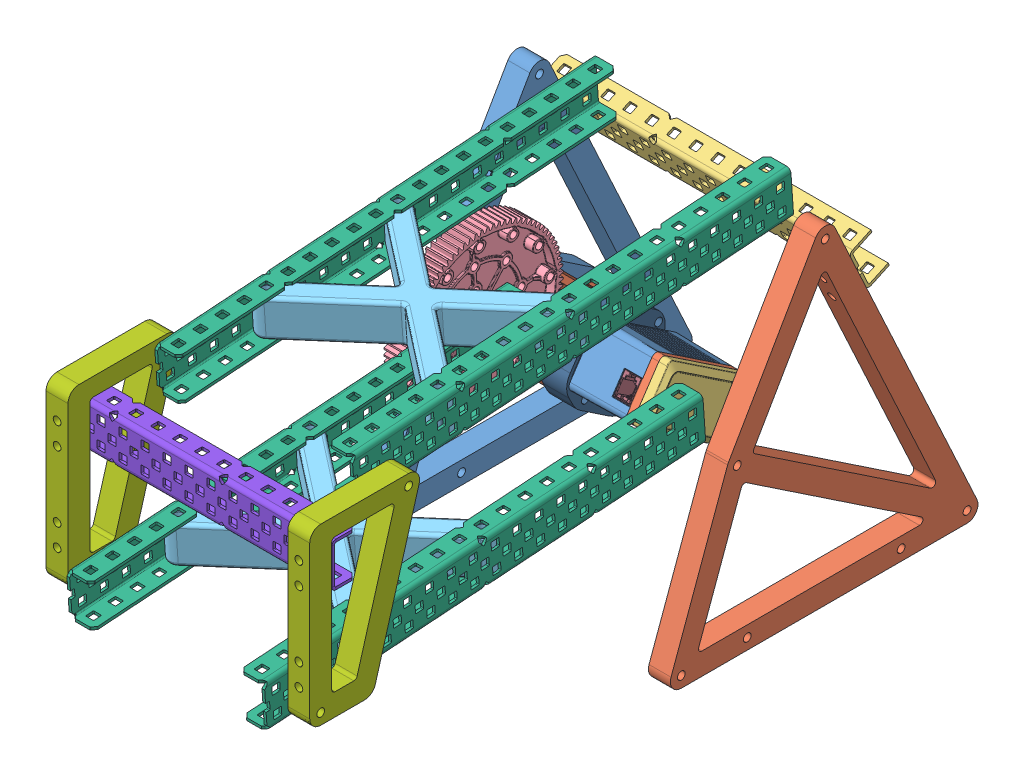
SolidWorks assembly RearArmAssembly, configuration Default. Lengths in mm.
43 component instances, 23 part files, 28 mates.
Components (placement in the parent):
- ArmMount-1: ArmMount [Default] at (3.0815 119.4615 170.9285) size (12.7 189.78 177.8)
- ArmMount(mirror)-1: ArmMount(mirror) [Default] at (168.1815 119.4615 170.9285) size (12.7 189.78 177.8)
- 1x2x1x14 Aluminum C-Channel-1: 1x2x1x14 Aluminum C-Channel [Default] at (225.3315 181.5036 101.1108) x (1 0 0) z (0 -0.420336 0.907368) size (177.8 25.41 13.97)
- RearArm_BottomBar-1: RearArm_BottomBar [Default] at (222.7102 54.1717 183.8088) x (0 -0.069828 0.997559) z (-1 0 0) size (286.79 90.98 127)
  - 84T High Strength Gear (276-3438)-1: 84T High Strength Gear (276-3438) [Default] at (-17.4079 64.2311 194.2288) size (90.98 90.98 12.7)
  - ArmXBrace-1: ArmXBrace [Default] at (128.6421 53.1059 130.7288) x (0 0 1) z (-1 0 0) size (111.86 22.25 88.94)
  - 1x2x1x20 Aluminum C-Channel-1: 1x2x1x20 Aluminum C-Channel [Default] at (192.1421 64.2311 187.8788) size (254 25.41 13.97)
  - 1x2x1x20 Aluminum C-Channel-2: 1x2x1x20 Aluminum C-Channel [Default] at (192.1421 64.2311 73.5788) x (1 0 0) z (0 0 -1) size (254 25.41 13.97)
- RearArm_TopBar-1: RearArm_TopBar [Default] at (12.5514 278.2747 177.0234) x (0 -0.069828 0.997559) z (1 0 0) size (254 25.4 114.31)
  - ArmXBrace-1: ArmXBrace [Default] at (94.2395 63.4998 79.4301) x (0 0 1) z (-1 0 0) size (111.86 22.25 88.94)
  - 1x2x1x20 Aluminum C-Channel-1: 1x2x1x20 Aluminum C-Channel [Default] at (157.7395 74.625 136.5801) size (254 25.41 13.97)
  - 1x2x1x20 Aluminum C-Channel-2: 1x2x1x20 Aluminum C-Channel [Default] at (157.7395 74.625 22.2801) x (1 0 0) z (0 0 -1) size (254 25.41 13.97)
- ArmEndAssembly-1: ArmEndAssembly [Default] at (208.3285 70.3449 488.0787) x (-1 0 0) z (0 0 -1) size (152.48 100.69 63.5)
  - ArmEnd-1: ArmEnd [Default] at (40.147 33.1539 89.1082) size (12.7 100.69 63.5)
  - ArmEnd-2: ArmEnd [Default] at (179.847 33.1539 89.1082) size (12.7 100.69 63.5)
  - 1x2x1x12 Aluminum C-Channel-1: 1x2x1x12 Aluminum C-Channel [Default] at (262.3169 103.0039 95.4582) x (1 0 0) z (0 0 -1) size (152.4 25.41 13.97)
- 0.5in 0.375in OD Nylon Spacer-1: 0.5in 0.375in OD Nylon Spacer [Default] at (22.1315 87.6603 123.4437) x (0 1 0) z (0 0 1) size (9.53 12.7 9.53)
- ArmMotorMount-1: ArmMotorMount [Default] at (41.1815 87.6603 123.4437) x (0 0.830879 -0.556452) z (1 0 0) size (48.1 53.1 15)
- 1.00_ Standoff (275-1016)-1: 1.00_ Standoff (275-1016) [Default] at (28.4815 71.832 134.0442) x (0 -1 0) z (0 0 1) size (7.34 25.4 7.34)
- 1.00_ Standoff (275-1016)-2: 1.00_ Standoff (275-1016) [Default] at (28.4815 103.4885 112.8433) x (0 -1 0) z (0 0 1) size (7.34 25.4 7.34)
- 1.00_ Standoff (275-1016)-3: 1.00_ Standoff (275-1016) [Default] at (28.4815 57.6981 112.9398) x (0 -1 0) z (0 0 1) size (7.34 25.4 7.34)
- 1.00_ Standoff (275-1016)-4: 1.00_ Standoff (275-1016) [Default] at (28.4815 89.3546 91.739) x (0 -1 0) z (0 0 1) size (7.34 25.4 7.34)
- V5 Smart Motor (276-4840) no cap-1: V5 Smart Motor (276-4840) no cap [Default] at (73.3815 80.5933 112.8916) x (0 0.556452 0.830879) z (-1 0 0) size (59.01 35.33 59.91)
  - V5 Smart Motor (276-4840).step-1: V5 Smart Motor (276-4840).step [Default] at origin size (59.01 35.33 59.91)
    - 276-4840-900 Rev6_Instruction.step-1: 276-4840-900 Rev6_Instruction.step [Default] at (-14.3 0 -17.2) size (52.79 15.94 38.15)
      - 276-4840-901 Rev6.step-1: 276-4840-901 Rev6.step [Default] at (10.75 -10.05 17.8) x (-1 0 0) z (0 0 1) size (49.9 1.6 38.15)
      - 276-4840-902 Rev2.step-1: 276-4840-902 Rev2.step [Default] at (31.25 -9.25 6.2) x (0 0 -1) z (0 -1 0) size (10.35 11.39 15.94)
      - 276-4840-022 Rev4.step-1: 276-4840-022 Rev4.step [Default] at (31.25 -9.25 6.2) x (0 0 -1) z (1 0 0) size (10.26 9.1 5.51)
    - 276-4840-110 Rev10_Instruction.step-1: 276-4840-110 Rev10_Instruction.step [Default] at (12.7 0 14.7) size (35.33 35.33 31.1)
      - 276-4840-061 Rev7_Ring_Gear_Fixed01 .6 Rev3.step-1: 276-4840-061 Rev7_Ring_Gear_Fixed01 .6 Rev3.step [Default] at origin size (28.79 28.39 24.6)
      - 276-4840-018 Rev6.step-1: 276-4840-018 Rev6.step [Default] at (0 0 6.7) x (-0.483174 0.875524 0) z (0 0 1) size (26 26 12.3)
      - 276-4840-059 Rev2.step-1: 276-4840-059 Rev2.step [Default] at (0 0 10.3) size (28.4 28.4 8.5)
      - 276-4840-062 Rev1.step-1: 276-4840-062 Rev1.step [Default] at (-12.1353 8.8168 12.3) x (0.956835 -0.290632 0) z (-0.290632 -0.956835 0) size (3.2 6.56 3.2)
      - 276-4840-062 Rev1.step-2: 276-4840-062 Rev1.step [Default] at (12.1353 8.8168 12.3) x (0.978427 0.206591 0) z (0.206591 -0.978427 0) size (3.2 6.56 3.2)
      - 276-4840-062 Rev1.step-3: 276-4840-062 Rev1.step [Default] at (-12.1353 -8.8168 12.3) x (0.72563 0.688086 0) z (0.688086 -0.72563 0) size (3.2 6.56 3.2)
    - 276-4840-001 Rev38.step-1: 276-4840-001 Rev38.step [Default] at origin size (57.3 33 46.9)
    - 276-4840-005 Rev27.step-1: 276-4840-005 Rev27.step [Default] at (0 0 -17.95) size (56.17 31.87 12.9)
    - 276-4840-004 Rev16.step-1: 276-4840-004 Rev16.step [Default] at (0 0 -19.2) size (56.01 31.71 9.21)
    - 276-4840-009 Rev3.step-1: 276-4840-009 Rev3.step [Default] at (25.45 13.5 15.7) x (0.19987 -0.979823 0) z (-0.979823 -0.19987 0) size (3.4 41.31 4.34)
    - 276-4840-009 Rev3.step-2: 276-4840-009 Rev3.step [Default] at (-25.45 -13.5 15.7) x (-0.998855 0.047836 0) z (0.047836 0.998855 0) size (3.4 41.31 4.34)
    - 276-4840-009 Rev3.step-3: 276-4840-009 Rev3.step [Default] at (25.45 -13.5 15.7) x (-0.975374 0.220559 0) z (0.220559 0.975374 0) size (3.4 41.31 4.34)
    - 276-4840-009 Rev3.step-4: 276-4840-009 Rev3.step [Default] at (-25.45 13.5 15.7) x (-0.922256 0.38658 0) z (0.38658 0.922256 0) size (3.4 41.31 4.34)
    - 276-4840-025 Rev19.step-1: 276-4840-025 Rev19.step [Default] at (12.7 0 -22.63) x (-0.993315 0.115437 0) z (0 0 1) size (14.82 14.83 35.18)
Mates (geometry in assembly coordinates):
- Concentric1: concentric aligned: cylinder of ArmMount-1 through (15.7815 30.5615 203.2855) axis (-1 0 0) radius 2.25; cylinder of ArmMount(mirror)-1 through (180.8815 30.5615 203.2855) axis (-1 0 0) radius 2.25
- Concentric2: concentric aligned: cylinder of ArmMount-1 through (15.7815 30.5615 165.1855) axis (-1 0 0) radius 2.25; cylinder of ArmMount(mirror)-1 through (180.8815 30.5615 165.1855) axis (-1 0 0) radius 2.25
- Coincident2: coincident anti-aligned: plane of ArmMount-1 through (15.7815 24.2115 28.2456) normal (0 0.420336 -0.907368); plane of 1x2x1x14 Aluminum C-Channel-1 through (3.5815 161.6138 91.8969) normal (0 -0.420336 0.907368)
- Concentric5: concentric anti-aligned: cylinder of ArmMount-1 through (9.4315 118.0828 253.1226) axis (0 0.420336 -0.907368) radius 2.25; circle of 1x2x1x14 Aluminum C-Channel-1
- Concentric6: concentric anti-aligned: cylinder of ArmMount(mirror)-1 through (174.5315 118.0828 253.1226) axis (0 0.420336 -0.907368) radius 2.25; circle of 1x2x1x14 Aluminum C-Channel-1
- Concentric11: concentric aligned: cylinder of ArmMount-1 through (15.7815 119.4615 170.9285) axis (-1 0 0) radius 2.25; circle of RearArm_BottomBar-1/1x2x1x20 Aluminum C-Channel-1
- Distance4: distance = 19.05 mm anti-aligned: plane of RearArm_BottomBar-1/1x2x1x20 Aluminum C-Channel-1 through (34.8315 98.4466 157.2276) normal (-1 0 0); plane of ArmMount-1 through (15.7815 119.4615 170.9285) normal (1 0 0)
- Distance5: distance = 19.05 mm anti-aligned: plane of RearArm_TopBar-1/1x2x1x20 Aluminum C-Channel-2 through (34.8315 186.4348 106.4276) normal (-1 0 0); plane of ArmMount-1 through (15.7815 119.4615 170.9285) normal (1 0 0)
- Concentric14: concentric anti-aligned: circle of RearArm_BottomBar-1/1x2x1x20 Aluminum C-Channel-1; cylinder of ArmEndAssembly-1/ArmEnd-2 through (15.7815 103.4989 398.9705) axis (1 0 0) radius 2.25
- Distance6: distance = 6.35 mm anti-aligned: plane of RearArm_BottomBar-1/1x2x1x20 Aluminum C-Channel-1 through (34.8315 98.4466 157.2276) normal (-1 0 0); plane of ArmEndAssembly-1/ArmEnd-2 through (28.4815 103.4989 398.9705) normal (1 0 0)
- Concentric15: concentric aligned: cylinder of ArmMount-1 through (15.7815 207.4497 120.1285) axis (-1 0 0) radius 2.25; circle of RearArm_TopBar-1/1x2x1x20 Aluminum C-Channel-2
- Concentric16: concentric anti-aligned: circle of RearArm_TopBar-1/1x2x1x20 Aluminum C-Channel-2; cylinder of ArmEndAssembly-1/ArmEnd-2 through (15.7815 191.487 348.1705) axis (1 0 0) radius 2.25
- Coincident9: coincident anti-aligned: plane of ArmMount-1 through (9.4315 87.6603 123.4437) normal (1 0 0); plane of 0.5in 0.375in OD Nylon Spacer-1 through (9.4315 87.6603 123.4437) normal (-1 0 0)
- Concentric17: concentric aligned: cylinder of ArmMount-1 through (9.4315 87.6603 123.4437) axis (1 0 0) radius 4.7625; cylinder of 0.5in 0.375in OD Nylon Spacer-1 through (9.4315 87.6603 123.4437) axis (1 0 0) radius 4.7625
- Concentric20: concentric anti-aligned: cylinder of ArmMount-1 through (15.7815 89.3546 91.739) axis (-1 0 0) radius 2.25; cylinder of 1.00_ Standoff (275-1016)-4 through (15.7815 89.3546 91.739) axis (1 0 0) radius 2.0955
- Concentric21: concentric anti-aligned: cylinder of ArmMount-1 through (15.7815 57.6981 112.9398) axis (-1 0 0) radius 2.25; cylinder of 1.00_ Standoff (275-1016)-3 through (15.7815 57.6981 112.9398) axis (1 0 0) radius 2.0955
- Concentric22: concentric anti-aligned: cylinder of ArmMount-1 through (15.7815 103.4885 112.8433) axis (-1 0 0) radius 2.25; cylinder of 1.00_ Standoff (275-1016)-2 through (15.7815 103.4885 112.8433) axis (1 0 0) radius 2.0955
- Concentric23: concentric anti-aligned: cylinder of ArmMount-1 through (15.7815 71.832 134.0442) axis (-1 0 0) radius 2.25; cylinder of 1.00_ Standoff (275-1016)-1 through (15.7815 71.832 134.0442) axis (1 0 0) radius 2.0955
- Coincident11: coincident anti-aligned: plane of ArmMount-1 through (15.7815 119.4615 170.9285) normal (1 0 0); plane of 1.00_ Standoff (275-1016)-1 through (15.7815 73.6651 130.8692) normal (-1 0 0)
- Coincident12: coincident anti-aligned: plane of ArmMount-1 through (15.7815 119.4615 170.9285) normal (1 0 0); plane of 1.00_ Standoff (275-1016)-3 through (15.7815 59.5312 109.7648) normal (-1 0 0)
- Coincident13: coincident anti-aligned: plane of ArmMount-1 through (15.7815 119.4615 170.9285) normal (1 0 0); plane of 1.00_ Standoff (275-1016)-4 through (15.7815 91.1877 88.564) normal (-1 0 0)
- Coincident14: coincident anti-aligned: plane of ArmMount-1 through (15.7815 119.4615 170.9285) normal (1 0 0); plane of 1.00_ Standoff (275-1016)-2 through (15.7815 105.3216 109.6683) normal (-1 0 0)
- Coincident15: coincident anti-aligned: plane of ArmMotorMount-1 through (41.1815 87.6603 123.4437) normal (-1 0 0); plane of 1.00_ Standoff (275-1016)-4 through (41.1815 91.1877 88.564) normal (1 0 0)
- Concentric24: concentric anti-aligned: cylinder of ArmMotorMount-1 through (56.1815 103.4885 112.8433) axis (-1 0 0) radius 2.25; cylinder of 1.00_ Standoff (275-1016)-2 through (15.7815 103.4885 112.8433) axis (1 0 0) radius 2.0955
- Concentric28: concentric aligned: cylinder of ArmMotorMount-1 through (56.1815 73.5264 102.3394) axis (-1 0 0) radius 4.3; cone of V5 Smart Motor (276-4840) no cap-1/V5 Smart Motor (276-4840).step-1/276-4840-001 Rev38.step-1 through (43.6815 73.5264 102.3394) axis (-1 0 0)
- Coincident16: coincident anti-aligned: plane of ArmMotorMount-1 through (56.1815 87.6603 123.4437) normal (1 0 0); plane of V5 Smart Motor (276-4840) no cap-1/V5 Smart Motor (276-4840).step-1/276-4840-001 Rev38.step-1 through (56.1815 77.3725 84.8998) normal (-1 0 0)
- Parallel2: parallel aligned: line of ArmMotorMount-1 through (56.1815 104.7161 122.8531) axis (0 -0.556452 -0.830879); line of V5 Smart Motor (276-4840) no cap-1/V5 Smart Motor (276-4840).step-1/276-4840-001 Rev38.step-1 through (57.1815 108.242 124.5236) axis (0 -0.556452 -0.830879)
- Parallel3: parallel aligned: plane of ArmMount-1 through (15.7815 98.3572 185.0624) normal (0 -0.830879 0.556452); plane of ArmMotorMount-1 through (56.1815 67.6776 136.8264) normal (0 -0.830879 0.556452)
